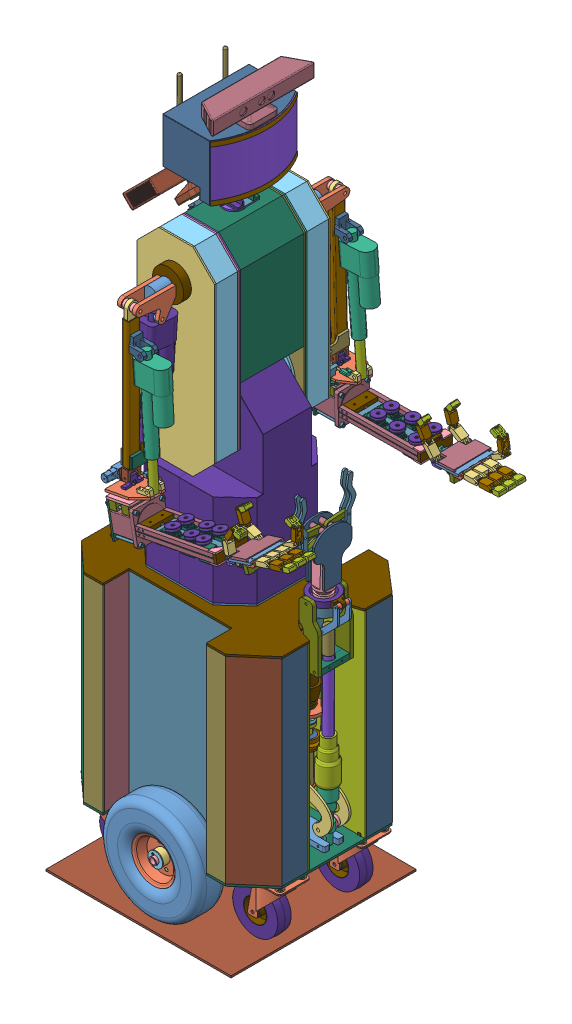
SolidWorks assembly sorbot, configuration По умолчанию. Lengths in mm. (continued)
Mates (geometry in assembly coordinates): (continued)
- Совпадение801: coincident anti-aligned: plane of ? through (-20.0648 1016.5246 -163.4875) normal (0 0 1); plane of body_tilt_axis_clamp-1 through (-20.0648 1016.5246 -163.4875) normal (0 0 -1)
- Концентричный435: concentric aligned: cylinder of body_axis-1 through (-20.0648 1016.5246 -50.7475) axis (0 0 -1) radius 10.9; cylinder of body_tilt_axis_clamp-2 through (-20.0648 1016.5246 -110.5942) axis (0 0 -1) radius 10.9
- Совпадение802: coincident anti-aligned: plane of ? through (-20.0648 1016.5246 -110.5942) normal (0 0 -1); plane of body_tilt_axis_clamp-2 through (-20.0648 1016.5246 -110.5942) normal (0 0 1)
- Концентричный436: concentric anti-aligned: cylinder of body_tilt_axis_clamp-1 through (-20.0648 1016.5246 -155.4875) axis (0 0 1) radius 20; cylinder of body_tilt_lever-1 through (-20.0648 1016.5246 -149.4875) axis (0 0 -1) radius 20
- Совпадение803: coincident anti-aligned: plane of body_tilt_axis_clamp-1 through (-20.0648 1016.5246 -155.4875) normal (0 0 1); plane of body_tilt_lever-1 through (-97.2168 978.7734 -155.4875) normal (0 0 -1)
- Заблокировать382: lock: unknown of ?; unknown of ?
- Заблокировать383: lock: unknown of ?; unknown of ?
- Заблокировать386: lock: unknown of ?; unknown of ?
- Заблокировать387: lock: unknown of ?; unknown of ?
- Заблокировать388: lock: unknown of body_pivot_fixture-1; unknown of body_pivot-2
- Заблокировать389: lock: unknown of ?; unknown of ?
- Заблокировать391: lock: unknown of body_pivot_fixture-1; unknown of ?
- Концентричный439: concentric aligned: cylinder of body_tilt_axis_clamp-2 through (-20.0648 1016.5246 -118.5942) axis (0 0 -1) radius 20; cylinder of body_tilt_lever-2 through (-20.0648 1016.5246 -118.5942) axis (0 0 -1) radius 20
- Концентричный440: concentric aligned: cylinder of body_tilt_lever-1 through (-99.3474 976.856 -149.4875) axis (0 0 -1) radius 5; cylinder of body_tilt_lever-2 through (-99.3474 976.856 -118.5942) axis (0 0 -1) radius 5
- Совпадение805: coincident anti-aligned: plane of body_tilt_axis_clamp-2 through (-20.0648 1016.5246 -118.5942) normal (0 0 -1); plane of body_tilt_lever-2 through (-97.2168 978.7734 -118.5942) normal (0 0 1)
- Концентричный441: concentric aligned: cylinder of body_tilt_lever-1 through (-99.3474 976.856 -149.4875) axis (0 0 -1) radius 5; cylinder of body_tilt_lever_axis-1 through (-99.3474 976.856 -80.4875) axis (0 0 -1) radius 5
- Расстояние22: distance = 40 mm aligned: plane of body_tilt_lever-1 through (-97.2168 978.7734 -155.4875) normal (0 0 -1); plane of body_tilt_lever_axis-1 through (-99.3474 976.856 -195.4875) normal (0 0 -1)
- Концентричный442: concentric anti-aligned: cylinder of body.tilit.lever.2-1 through (-99.3474 976.856 -188.4655) axis (0 0 1) radius 5; cylinder of body_tilt_lever_axis-1 through (-99.3474 976.856 -80.4875) axis (0 0 -1) radius 5
- Концентричный443: concentric anti-aligned: cylinder of tilt.thread.rod-1 through (-119.3768 928.5591 -141.6211) axis (0 1 0) radius 6; cylinder of body.tilt.nut-1 through (-119.3768 842.3995 -141.6211) axis (0 -1 0) radius 8
- Концентричный444: concentric anti-aligned: cylinder of tilt.thread.rod-1 through (-119.3768 928.5591 -141.6211) axis (0 1 0) radius 6; cylinder of body.tilit.nut.housing-1 through (-119.3768 838.3995 -141.6211) axis (0 -1 0) radius 8
- Концентричный445: concentric anti-aligned: cylinder of body.tilit.lever.2-1 through (-119.3768 828.3995 -188.4655) axis (0 0 1) radius 5; cylinder of body.tilit.nut.housing-1 through (-119.3768 828.3995 -156.4655) axis (0 0 -1) radius 5
- Концентричный446: concentric aligned: cylinder of body.tilit.nut.housing-1 through (-119.3768 828.3995 -156.4655) axis (0 0 -1) radius 5; cylinder of body.tilit.nut.housing.bolt-1 through (-119.3768 828.3995 -158.4655) axis (0 0 -1) radius 5
- Совпадение808: coincident anti-aligned: plane of body.tilt.nut-1 through (-110.3768 828.3995 -126.0327) normal (0 -1 0); plane of body.tilit.nut.housing-1 through (-94.3768 828.3995 -157.2211) normal (0 1 0)
- Параллельность198: parallel anti-aligned: plane of body.tilt.nut-1 through (-110.3768 842.3995 -157.2096) normal (0 0 -1); plane of body.tilit.nut.housing-1 through (-144.3768 828.3995 -157.2211) normal (0 0 1)
- Заблокировать392: lock: unknown of ?; unknown of ?
- Совпадение810: coincident anti-aligned: plane of body.tilit.lever.2-1 through (-119.3768 828.3995 -181.4655) normal (0 0 1); plane of body.tilit.nut.housing-1 through (-141.3638 838.3995 -181.4655) normal (0 0 -1)
- Совпадение811: coincident anti-aligned: plane of body.tilit.lever.2-1 through (-119.3768 828.3995 -188.4655) normal (0 0 -1); plane of body.tilit.nut.housing.bolt-1 through (-129.642 830.0202 -188.4655) normal (0 0 1)
- Концентричный447: concentric anti-aligned: cylinder of body_tilt_lever_axis-1 through (-99.3474 976.856 -80.4875) axis (0 0 -1) radius 5; cylinder of body.tilit.extender-1 through (-99.3474 976.856 -176.9875) axis (0 0 1) radius 5
- Совпадение812: coincident anti-aligned: plane of body_tilt_lever-1 through (-97.2168 978.7734 -155.4875) normal (0 0 -1); plane of body.tilit.extender-1 through (-99.3474 976.856 -155.4875) normal (0 0 1)
- Концентричный448: concentric aligned: cylinder of body_tilt_lever_axis-1 through (-99.3474 976.856 -80.4875) axis (0 0 -1) radius 5; cylinder of washer-1 through (-99.3474 976.856 -188.4655) axis (0 0 -1) radius 5
- Совпадение813: coincident anti-aligned: plane of body.tilit.lever.2-1 through (-119.3768 828.3995 -188.4655) normal (0 0 -1); plane of washer-1 through (-99.3474 976.856 -188.4655) normal (0 0 1)
- Концентричный449: concentric anti-aligned: cylinder of body_tilt_lever_axis-1 through (-99.3474 976.856 -80.4875) axis (0 0 -1) radius 5; cylinder of body.tilit.extender-2 through (-99.3474 976.856 -118.5942) axis (0 0 1) radius 5
- Совпадение814: coincident anti-aligned: plane of body_tilt_lever-2 through (-97.2168 978.7734 -118.5942) normal (0 0 1); plane of body.tilit.extender-2 through (-99.3474 976.856 -118.5942) normal (0 0 -1)
- Концентричный450: concentric anti-aligned: cylinder of body_tilt_lever_axis-1 through (-99.3474 976.856 -80.4875) axis (0 0 -1) radius 5; cylinder of body.tilit.lever.2-2 through (-99.3474 976.856 -101.7768) axis (0 0 1) radius 5
- Концентричный451: concentric aligned: cylinder of body.tilit.nut.housing-1 through (-119.3768 828.3995 -126.7768) axis (0 0 1) radius 5; cylinder of body.tilit.lever.2-2 through (-119.3768 828.3995 -101.7768) axis (0 0 1) radius 5
- Совпадение816: coincident anti-aligned: plane of body.tilit.nut.housing-1 through (-141.3638 838.3995 -101.7768) normal (0 0 1); plane of body.tilit.lever.2-2 through (-119.3768 828.3995 -101.7768) normal (0 0 -1)
- Концентричный452: concentric aligned: cylinder of body.tilit.nut.housing-1 through (-119.3768 828.3995 -126.7768) axis (0 0 1) radius 5; cylinder of body.tilit.nut.housing.bolt-2 through (-119.3768 828.3995 -124.7768) axis (0 0 1) radius 5
- Совпадение817: coincident anti-aligned: plane of body.tilit.lever.2-2 through (-119.3768 828.3995 -94.7768) normal (0 0 1); plane of body.tilit.nut.housing.bolt-2 through (-109.1117 830.0202 -94.7768) normal (0 0 -1)
- Концентричный453: concentric aligned: cylinder of body_tilt_lever_axis-1 through (-99.3474 976.856 -80.4875) axis (0 0 -1) radius 5; cylinder of washer-2 through (-99.3474 976.856 -92.7768) axis (0 0 -1) radius 5
- Совпадение818: coincident anti-aligned: plane of body.tilit.lever.2-2 through (-119.3768 828.3995 -94.7768) normal (0 0 1); plane of washer-2 through (-99.3474 976.856 -94.7768) normal (0 0 -1)
- Совпадение819: coincident anti-aligned: plane of body.frame.p1-3 through (92.5097 1436.2936 -50.7442) normal (0 0 -1); plane of arm.fixture.cap-1 through (-12.4559 1335.4922 -50.7442) normal (0 0 1)
- Совпадение820: coincident anti-aligned: plane of ? through (412.7357 1007.5295 110.4481) normal (-0.012247 -0.004016 0.999917); plane of finger.p2-10 through (405.8167 1000.5207 110.3352) normal (0.012247 0.004016 -0.999917)
- Заблокировать394: lock: unknown of ?; unknown of ?
- Заблокировать395: lock: unknown of ?; unknown of ?
- Заблокировать396: lock: unknown of ?; unknown of ?
- Заблокировать397: lock: unknown of ?; unknown of ?
- Заблокировать398: lock: unknown of ?; unknown of ?
- Заблокировать399: lock: unknown of ?; unknown of ?
- Заблокировать402: lock: unknown of ?; unknown of ?
- Заблокировать405: lock: unknown of ?; unknown of ?
- Концентричный459: concentric anti-aligned: cylinder of cap-hinge-p1-3 through (95.5097 1327.1115 -226.3787) axis (0 -1 0) radius 2; cylinder of cap-hinge-5 through (95.5097 1287.9494 -226.3787) axis (0 1 0) radius 2
- Совпадение845: coincident anti-aligned: plane of cap-hinge-p1-3 through (75.5097 1317.9494 -221.4356) normal (0 1 0); plane of cap-hinge-5 through (75.5404 1317.9494 -220.4411) normal (0 -1 0)
- Заблокировать404: lock: unknown of ?; unknown of ?
- Заблокировать406: lock: unknown of ?; unknown of ?
- Концентричный460: concentric anti-aligned: cylinder of cap-hinge-p1-4 through (95.5097 1143.936 -226.3787) axis (0 1 0) radius 2; cylinder of cap-hinge-4 through (95.5097 1183.1735 -226.3787) axis (0 -1 0) radius 2
- Совпадение847: coincident anti-aligned: plane of cap-hinge-4 through (75.5097 1173.1735 -232.2123) normal (0 -1 0); plane of cap-hinge-p1-4 through (75.4842 1173.1735 -231.2174) normal (0 1 0)
- Заблокировать407: lock: unknown of ?; unknown of ?
- Заблокировать410: lock: unknown of ?; unknown of ?
- Совпадение849: coincident anti-aligned: plane of body_pivot_fixture-1 through (-20.0648 937.0246 -136.9555) normal (0 -1 0); plane of tilit.thread.rod.bearing.fixture-1 through (-20.0648 937.0246 -136.9555) normal (0 1 0)
- Заблокировать411: lock: unknown of body_pivot_fixture-1; unknown of ?
- Параллельность199: parallel aligned: plane of wall6-3 through (267.1742 -18.2461 -216.2424) normal (1 0 0); plane of ? through (92.0581 957.5993 348.483) normal (1 0 0)
- Заблокировать412: lock: unknown of ?; unknown of ?
- Совпадение851: coincident anti-aligned: plane of body.frame.p4-4 through (-117.3772 1436.2936 -226.3595) normal (0 0 1); plane of shoulder.bearing.housing-4 through (-12.3772 1335.516 -226.3595) normal (0 0 -1)
- Концентричный462: concentric aligned: cylinder of body.frame.p4-4 through (-12.3772 1335.516 -226.3595) axis (0 0 -1) radius 12.5; cylinder of shoulder.bearing.housing-4 through (-12.3772 1335.516 -205.3595) axis (0 0 -1) radius 15.5
- Заблокировать413: lock: unknown of ?; unknown of ?
- Концентричный463: concentric aligned: cylinder of shoulder.bearing.housing-3 through (-12.6499 1335.3853 -313.3595) axis (0 0 1) radius 15.5; cylinder of shoulder.axis-2 through (-12.6499 1335.3853 -317.3595) axis (0 0 1) radius 15
- Совпадение853: coincident aligned: plane of shoulder.bearing.housing-4 through (-12.3772 1335.516 -205.3595) normal (0 0 1); plane of shoulder.axis-2 through (-12.6499 1335.3853 -205.3595) normal (0 0 1)
- Совпадение855: coincident: plane of body.frame.p4-4 through (-117.3772 1436.2936 -230.3595) normal (0 0 -1); plane of shoulder.p6-3
- Совпадение856: coincident anti-aligned: plane of shoulder.p6-4 through (-12.6499 1335.3853 -288.3595) normal (0 0 -1); plane of body.frame.p4.external-1 through (-117.6384 1436.1749 -288.3595) normal (0 0 1)
- Концентричный464: concentric aligned: cylinder of shoulder.axis-2 through (-12.6499 1335.3853 -317.3595) axis (0 0 1) radius 15; cylinder of shoulder.p6-3 through (-12.6499 1335.3853 -245.2739) axis (0 0 1) radius 15
- Концентричный465: concentric anti-aligned: cylinder of shoulder.axis-2 through (-12.6499 1335.3853 -317.3595) axis (0 0 1) radius 15; cylinder of shoulder.p6-4 through (-12.6499 1335.3853 -270.3595) axis (0 0 -1) radius 15
- Совпадение857: coincident: plane of ?; plane of shoulder.p4-3 through (-59.8188 1400.1357 -245.3595) normal (0 0 1)
- Совпадение858: coincident anti-aligned: plane of shoulder.p6-4 through (-12.6499 1335.3853 -270.3595) normal (0 0 1); plane of shoulder.p4-4 through (-59.8188 1400.1357 -270.3595) normal (0 0 -1)
- Концентричный466: concentric anti-aligned: cylinder of shoulder.axis-2 through (-12.6499 1335.3853 -317.3595) axis (0 0 1) radius 15; cylinder of shoulder.p4-4 through (-12.6499 1335.3853 -266.3595) axis (0 0 -1) radius 15
- Концентричный467: concentric anti-aligned: cylinder of shoulder.axis-2 through (-12.6499 1335.3853 -317.3595) axis (0 0 1) radius 15; cylinder of shoulder.p4-3 through (-12.6499 1335.3853 -245.3595) axis (0 0 -1) radius 15
- Совпадение865: coincident anti-aligned: plane of body.frame.p4-4 through (-117.3772 1436.2936 -230.3595) normal (0 0 -1); plane of arm.lift.actuator.fixture.p3-3 through (-88.5702 993.1387 -230.3595) normal (0 0 1)
- Концентричный469: concentric aligned: cylinder of arm.lift.actuator.fixture.p3-3 through (-88.5702 993.1387 -230.3595) axis (0 0 -1) radius 4; cylinder of arm.lift.actuator.fixture.p2-2 through (-88.5702 993.1387 -230.3595) axis (0 0 -1) radius 4
- Заблокировать416: lock: unknown of ?; unknown of ?
- Заблокировать415: lock: unknown of ?; unknown of ?
- Концентричный470: concentric anti-aligned: cylinder of arm.lift.actuator.fixture.p3-4 through (-88.5702 993.1387 -288.3595) axis (0 0 1) radius 4; cylinder of arm.lift.actuator.fixture.p2-2 through (-88.5702 993.1387 -230.3595) axis (0 0 -1) radius 4
- Концентричный478: concentric aligned: cylinder of arm.lift.actuator.fixture.p2-2 through (-88.5702 993.1387 -230.3595) axis (0 0 -1) radius 4; cylinder of arm.actuator-4/arm.actuator.p1-1 through (-88.5702 993.1387 -244.3595) axis (0 0 -1) radius 4.1
- Касательный33: tangent anti-aligned: plane of arm.lift.actuator.fixture.p3-3 through (-88.5702 993.1387 -249.3595) normal (0 0 -1); cylinder of arm.actuator-4/arm.actuator.p1-1 through (-89.1112 985.157 -259.3595) axis (0.067628 0.997711 0) radius 10
- Концентричный480: concentric anti-aligned: cylinder of arm.actuator-4/arm.actuator.p1-1 through (-79.508 1126.8319 -259.3595) axis (0.067628 0.997711 0) radius 10; cylinder of arm.actuator.p2-4 through (-60.3086 1410.0778 -259.3595) axis (-0.067628 -0.997711 0) radius 10
- Концентричный482: concentric anti-aligned: cylinder of shoulder.p4-4 through (-60.8835 1401.5972 -266.3595) axis (0 0 -1) radius 4; cylinder of arm.actuator.p2-4 through (-60.8835 1401.5972 -284.3595) axis (0 0 1) radius 4
- Концентричный481: concentric anti-aligned: cylinder of shoulder.p4-3 through (-60.8835 1401.5972 -245.3595) axis (0 0 -1) radius 4; cylinder of arm.actuator.p2-4 through (-60.8835 1401.5972 -284.3595) axis (0 0 1) radius 4
- Заблокировать418: lock: unknown of ?; unknown of ?
- Заблокировать419: lock: unknown of ?; unknown of ?
- Концентричный483: concentric anti-aligned: cylinder of arm.fixture-4 through (2.8485 1335.3868 -413.2628) axis (0.999986 0 0.005196) radius 4; cylinder of arm.lift2.actuator.fixture.p1-4 through (2.8485 1335.3868 -413.2628) axis (-0.999986 0 -0.005196) radius 4
- Совпадение869: coincident anti-aligned: plane of arm.fixture-4 through (2.8437 1335.375 -412.3468) normal (-0.999986 0 -0.005196); plane of arm.lift2.actuator.fixture.p1-4 through (2.8485 1335.3868 -413.2628) normal (0.999986 0 0.005196)
- Заблокировать420: lock: unknown of ?; unknown of ?
- Концентричный484: concentric aligned: cylinder of shoulder.lever-2 through (-7.1514 1335.3868 -413.3148) axis (-0.999986 0 -0.005196) radius 4; cylinder of arm.lift2.actuator.fixture.p1-4 through (2.8485 1335.3868 -413.2628) axis (-0.999986 0 -0.005196) radius 4
- Совпадение870: coincident anti-aligned: plane of shoulder.lever-2 through (-7.1514 1335.3868 -413.3154) normal (0.999986 0 0.005196); plane of arm.lift2.actuator.fixture.p1-4 through (-7.1514 1335.3868 -413.3148) normal (-0.999986 0 -0.005196)
- Концентричный485: concentric anti-aligned: cylinder of arm.fixture-5 through (-37.1514 1335.3868 -413.3148) axis (0.999986 0 0.005196) radius 4; cylinder of arm.lift2.actuator.fixture.p1-5 through (-17.1517 1335.3868 -413.2109) axis (-0.999986 0 -0.005196) radius 4
- Совпадение871: coincident anti-aligned: plane of arm.fixture-5 through (-27.1563 1335.375 -412.3468) normal (0.999986 0 0.005196); plane of arm.lift2.actuator.fixture.p1-5 through (-27.1515 1335.3868 -413.2628) normal (-0.999986 0 -0.005196)
- Заблокировать422: lock: unknown of ?; unknown of ?
- Концентричный486: concentric anti-aligned: cylinder of arm.fixture-4 through (2.5373 1286.6879 -353.3754) axis (0.999986 0 0.005196) radius 4; cylinder of arm.actuator-5/arm.actuator.p1-1 through (2.5373 1286.6879 -353.3754) axis (-0.999986 0 -0.005196) radius 4.1
- Концентричный487: concentric anti-aligned: cylinder of arm.fixture-4 through (2.5373 1286.6879 -353.3754) axis (0.999986 0 0.005196) radius 4; cylinder of arm.lift2.actuator.fixture.p1.m1-3 through (2.5373 1286.6879 -353.3754) axis (-0.999986 0 -0.005196) radius 4
- Совпадение873: coincident anti-aligned: plane of arm.fixture-4 through (2.8437 1335.375 -412.3468) normal (-0.999986 0 -0.005196); plane of arm.lift2.actuator.fixture.p1.m1-3 through (2.5373 1286.6879 -353.3754) normal (0.999986 0 0.005196)
- Концентричный488: concentric anti-aligned: cylinder of arm.fixture-5 through (-37.4626 1286.6879 -353.4274) axis (0.999986 0 0.005196) radius 4; cylinder of arm.lift2.actuator.fixture.p1.m1-4 through (-22.4628 1286.6879 -353.3495) axis (-0.999986 0 -0.005196) radius 4
- Совпадение874: coincident anti-aligned: plane of arm.fixture-5 through (-27.1563 1335.375 -412.3468) normal (0.999986 0 0.005196); plane of arm.lift2.actuator.fixture.p1.m1-4 through (-27.4627 1286.6879 -353.3754) normal (-0.999986 0 -0.005196)
- Касательный34: tangent anti-aligned: cylinder of arm.actuator-5/arm.actuator.p1-1 through (-12.4664 1294.6528 -352.7052) axis (0.000486 -0.995617 -0.093518) radius 10; plane of arm.lift2.actuator.fixture.p1.m1-3 through (-2.4627 1286.6879 -353.4014) normal (-0.999986 0 -0.005196)
- Заблокировать423: lock: unknown of ?; unknown of ?
- Заблокировать424: lock: unknown of ?; unknown of ?
- Заблокировать425: lock: unknown of ?; unknown of ?
- Заблокировать426: lock: unknown of ?; unknown of ?
- Заблокировать427: lock: unknown of ?; unknown of ?
- Заблокировать428: lock: unknown of ?; unknown of ?
- Заблокировать429: lock: unknown of ?; unknown of ?
- Заблокировать430: lock: unknown of ?; unknown of ?
- Концентричный493: concentric aligned: cylinder of actuator.100.fixture-2 through (30.5425 1248.8767 -435.037) axis (-0.005195 -0.022106 0.999742) radius 4; cylinder of arm.actuator100mm..p1-2 through (30.516 1248.7636 -429.924) axis (-0.005195 -0.022106 0.999742) radius 4
- Касательный35: tangent anti-aligned: plane of actuator.100.fixture-2 through (40.8098 1209.6631 -405.7286) normal (0.005195 0.022106 -0.999742); cylinder of arm.actuator100mm..p1-2 through (29.9802 1256.417 -414.7536) axis (0.057231 -0.998124 -0.021773) radius 10
- Концентричный495: concentric anti-aligned: cylinder of arm.actuator100mm..p1-2 through (35.3599 1162.5934 -416.8003) axis (0.057231 -0.998124 -0.021773) radius 10; cylinder of arm.actuator100mm.p2-2 through (49.2611 920.154 -422.0889) axis (-0.057231 0.998124 0.021773) radius 10
- Заблокировать445: lock: unknown of ?; unknown of ?
- Заблокировать446: lock: unknown of ?; unknown of ?
- Заблокировать447: lock: unknown of ?; unknown of ?
- Заблокировать448: lock: unknown of ?; unknown of ?
- Заблокировать449: lock: unknown of ?; unknown of ?
- Заблокировать450: lock: unknown of ?; unknown of ?
- Заблокировать451: lock: unknown of ?; unknown of ?
- Концентричный504: concentric anti-aligned: cylinder of HS-311 Hitec Standard Servo and Horn-12/HS-311-p2-1 through (110.806 865.1228 -440.1318) axis (-0.012385 0.99968 0.022041) radius 4.064; cylinder of lower.arm.p9-8 through (110.7286 871.3708 -439.994) axis (0.012385 -0.99968 -0.022041) radius 12
- Концентричный505: concentric anti-aligned: cylinder of HS-311 Hitec Standard Servo and Horn-8/HS-311-p2-1 through (165.824 865.856 -442.4703) axis (-0.012385 0.99968 0.022041) radius 4.064; cylinder of lower.arm.p9-10 through (165.7466 872.104 -442.3326) axis (0.012385 -0.99968 -0.022041) radius 12
- Концентричный506: concentric anti-aligned: cylinder of HS-311 Hitec Standard Servo and Horn-10/HS-311-p2-1 through (220.8415 866.5874 -444.7289) axis (-0.012385 0.99968 0.022041) radius 4.064; cylinder of lower.arm.p9-12 through (220.7641 872.8354 -444.5912) axis (0.012385 -0.99968 -0.022041) radius 12
- Концентричный507: concentric anti-aligned: cylinder of HS-311 Hitec Standard Servo and Horn-11/HS-311-p2-1 through (110.6228 864.3429 -404.8609) axis (-0.012385 0.99968 0.022041) radius 4.064; cylinder of lower.arm.p9-7 through (110.5453 870.5909 -404.7231) axis (0.012385 -0.99968 -0.022041) radius 12
- Концентричный508: concentric anti-aligned: cylinder of HS-311 Hitec Standard Servo and Horn-7/HS-311-p2-1 through (165.6133 864.9593 -401.9208) axis (-0.012385 0.99968 0.022041) radius 4.064; cylinder of lower.arm.p9-9 through (165.5359 871.2073 -401.783) axis (0.012385 -0.99968 -0.022041) radius 12
- Концентричный509: concentric anti-aligned: cylinder of HS-311 Hitec Standard Servo and Horn-9/HS-311-p2-1 through (220.6042 865.5775 -399.0607) axis (-0.012385 0.99968 0.022041) radius 4.064; cylinder of lower.arm.p9-11 through (220.5268 871.8255 -398.923) axis (0.012385 -0.99968 -0.022041) radius 12
- Совпадение938: coincident anti-aligned: plane of HS-311 Hitec Standard Servo and Horn-12/HS-311-p2-1 through (112.9596 871.5833 -448.3789) normal (-0.012385 0.99968 0.022041); plane of lower.arm.p9-8 through (110.7286 871.3708 -439.994) normal (0.012385 -0.99968 -0.022041)
- Совпадение939: coincident anti-aligned: plane of HS-311 Hitec Standard Servo and Horn-8/HS-311-p2-1 through (167.9775 872.3165 -450.7175) normal (-0.012385 0.99968 0.022041); plane of lower.arm.p9-10 through (165.7466 872.104 -442.3326) normal (0.012385 -0.99968 -0.022041)
- Совпадение940: coincident anti-aligned: plane of HS-311 Hitec Standard Servo and Horn-10/HS-311-p2-1 through (222.9951 873.0479 -452.9761) normal (-0.012385 0.99968 0.022041); plane of lower.arm.p9-12 through (220.7641 872.8354 -444.5912) normal (0.012385 -0.99968 -0.022041)
- Совпадение941: coincident anti-aligned: plane of HS-311 Hitec Standard Servo and Horn-9/HS-311-p2-1 through (222.7577 872.038 -407.3079) normal (-0.012385 0.99968 0.022041); plane of lower.arm.p9-11 through (220.5268 871.8255 -398.923) normal (0.012385 -0.99968 -0.022041)
- Совпадение942: coincident anti-aligned: plane of HS-311 Hitec Standard Servo and Horn-7/HS-311-p2-1 through (167.7668 871.4198 -410.168) normal (-0.012385 0.99968 0.022041); plane of lower.arm.p9-9 through (165.5359 871.2073 -401.783) normal (0.012385 -0.99968 -0.022041)
- Совпадение943: coincident anti-aligned: plane of HS-311 Hitec Standard Servo and Horn-11/HS-311-p2-1 through (112.7763 870.8034 -413.108) normal (-0.012385 0.99968 0.022041); plane of lower.arm.p9-7 through (110.5453 870.5909 -404.7231) normal (0.012385 -0.99968 -0.022041)
- Заблокировать452: lock: unknown of ?; unknown of ?
- Заблокировать453: lock: unknown of ?; unknown of ?
- Заблокировать454: lock: unknown of ?; unknown of ?
- Заблокировать455: lock: unknown of ?; unknown of ?
- Заблокировать456: lock: unknown of ?; unknown of ?
- Заблокировать458: lock: unknown of ?; unknown of ?
- Совпадение963: coincident anti-aligned: plane of palm.p1-4 through (362.2803 874.0257 -470.765) normal (-0.060104 0.997955 0.021755); plane of palm.p6-3 through (295.9379 868.6488 -407.401) normal (0.060104 -0.997955 -0.021755)
- Совпадение964: coincident anti-aligned: plane of palm.p1-4 through (362.2803 874.0257 -470.765) normal (-0.060104 0.997955 0.021755); plane of palm.p6-4 through (296.3955 869.3003 -436.0217) normal (0.060104 -0.997955 -0.021755)
- Совпадение965: coincident anti-aligned: plane of palm.p1-4 through (362.2803 874.0257 -470.765) normal (-0.060104 0.997955 0.021755); plane of palm.p5-3 through (330.0768 870.2924 -388.4794) normal (0.060104 -0.997955 -0.021755)
- Совпадение966: coincident anti-aligned: plane of palm.p1-4 through (362.2803 874.0257 -470.765) normal (-0.060104 0.997955 0.021755); plane of palm.p5-4 through (330.5285 871.7398 -453.6282) normal (0.060104 -0.997955 -0.021755)
- Заблокировать459: lock: unknown of ?; unknown of ?
- Заблокировать460: lock: unknown of ?; unknown of ?
- Заблокировать461: lock: unknown of ?; unknown of ?
- Заблокировать462: lock: unknown of ?; unknown of ?
- Совпадение967: coincident anti-aligned: plane of palm.p1-4 through (362.2803 874.0257 -470.765) normal (-0.060104 0.997955 0.021755); plane of palm.cap-2 through (306.1449 870.1321 -447.243) normal (0.060104 -0.997955 -0.021755)
- Совпадение968: coincident aligned: plane of palm.p1-4 through (286.8974 867.3169 -371.2793) normal (-0.998179 -0.059975 -0.006513); plane of palm.cap-2 through (286.6609 873.8329 -395.0363) normal (-0.998179 -0.059975 -0.006513)
- Совпадение969: coincident aligned: plane of palm.p1-4 through (286.8974 867.3169 -371.2793) normal (-0.005195 -0.022106 0.999742); plane of palm.cap-2 through (349.3088 877.0763 -370.7392) normal (-0.005195 -0.022106 0.999742)
- Заблокировать463: lock: unknown of ?; unknown of ?
- Совпадение970: coincident anti-aligned: plane of palm.p1-4 through (362.641 868.038 -470.8956) normal (0.060104 -0.997955 -0.021755); plane of palm.p3.m-3 through (319.6212 863.2737 -371.1987) normal (-0.060104 0.997955 0.021755)
- Совпадение971: coincident aligned: plane of palm.p1-4 through (286.8974 867.3169 -371.2793) normal (-0.005195 -0.022106 0.999742); plane of palm.p3.m-3 through (287.7592 869.3718 -371.2294) normal (-0.005195 -0.022106 0.999742)
- Совпадение972: coincident anti-aligned: plane of palm.p1-4 through (296.9 868.0051 -375.2131) normal (-0.998179 -0.059975 -0.006513); plane of palm.p3.m-3 through (296.6978 870.9282 -371.1485) normal (0.998179 0.059975 0.006513)
- Заблокировать464: lock: unknown of ?; unknown of ?
- Совпадение973: coincident anti-aligned: plane of palm.p1-4 through (362.641 868.038 -470.8956) normal (0.060104 -0.997955 -0.021755); plane of palm.p3.m-4 through (320.029 865.0091 -449.6784) normal (-0.060104 0.997955 0.021755)
- Совпадение974: coincident aligned: plane of palm.p1-4 through (287.4169 869.5276 -471.2535) normal (0.005195 0.022106 -0.999742); plane of palm.p3.m-4 through (288.2787 871.5825 -471.2036) normal (0.005195 0.022106 -0.999742)
- Совпадение975: coincident anti-aligned: plane of palm.p1-4 through (297.3779 870.0389 -467.1894) normal (-0.998179 -0.059975 -0.006513); plane of palm.p3.m-4 through (297.1057 872.6635 -449.6283) normal (0.998179 0.059975 0.006513)
- Заблокировать465: lock: unknown of ?; unknown of ?
- Совпадение976: coincident anti-aligned: plane of palm.p1-4 through (362.641 868.038 -470.8956) normal (0.060104 -0.997955 -0.021755); plane of palm.p3-2 through (343.569 866.8921 -471.02) normal (-0.060104 0.997955 0.021755)
- Совпадение977: coincident aligned: plane of palm.p1-4 through (286.8974 867.3169 -371.2793) normal (-0.005195 -0.022106 0.999742); plane of palm.p3-2 through (370.5503 875.8487 -370.6559) normal (-0.005195 -0.022106 0.999742)
- Совпадение978: coincident anti-aligned: plane of palm.p1-4 through (361.7608 871.8151 -370.7908) normal (0.998179 0.059975 0.006513); plane of palm.p3-2 through (362.07 877.5186 -470.6889) normal (-0.998179 -0.059975 -0.006513)
- Заблокировать466: lock: unknown of ?; unknown of ?
- Концентричный510: concentric aligned: cylinder of palm.p3.m-3 through (292.5129 865.4279 -371.2919) axis (0.005195 0.022106 -0.999742) radius 1.5; cylinder of finger.p1-7 through (292.5155 865.439 -371.7918) axis (0.005195 0.022106 -0.999742) radius 1.5
- Совпадение979: coincident anti-aligned: plane of palm.p3.m-3 through (282.5498 857.4215 -389.0252) normal (-0.005195 -0.022106 0.999742); plane of finger.p1-7 through (295.546 853.9979 -389.0334) normal (0.005195 0.022106 -0.999742)
- Концентричный512: concentric aligned: cylinder of finger.p2-13 through (267.069 896.9455 -371.2273) axis (0.005195 0.022106 -0.999742) radius 1.5; cylinder of finger.p1-7 through (267.069 896.9455 -371.2273) axis (0.005195 0.022106 -0.999742) radius 1.5
- Совпадение980: coincident anti-aligned: plane of finger.p1-7 through (268.2587 888.6357 -387.9091) normal (-0.005195 -0.022106 0.999742); plane of finger.p2-13 through (268.1702 885.8361 -387.9715) normal (0.005195 0.022106 -0.999742)
- Концентричный513: concentric aligned: cylinder of finger.p2-13 through (248.7323 931.3594 -370.5616) axis (0.005195 0.022106 -0.999742) radius 1.5; cylinder of finger.p3-7 through (248.7328 931.3619 -370.6745) axis (0.005195 0.022106 -0.999742) radius 1.5
- Совпадение981: coincident anti-aligned: plane of finger.p2-13 through (248.3728 922.9913 -387.2528) normal (-0.005195 -0.022106 0.999742); plane of finger.p3-7 through (238.9673 925.751 -387.2406) normal (0.005195 0.022106 -0.999742)
- Заблокировать467: lock: unknown of ?; unknown of ?
- Заблокировать468: lock: unknown of ?; unknown of ?
- Заблокировать469: lock: unknown of ?; unknown of ?
- Концентричный514: concentric aligned: cylinder of palm.p3.m-4 through (292.9207 867.1633 -449.7716) axis (0.005195 0.022106 -0.999742) radius 1.5; cylinder of finger.p1-8 through (292.9233 867.1743 -450.2715) axis (0.005195 0.022106 -0.999742) radius 1.5
- Совпадение982: coincident anti-aligned: plane of palm.p3.m-4 through (282.9576 859.1568 -467.505) normal (-0.005195 -0.022106 0.999742); plane of ? through (299.5757 857.2919 -467.4599) normal (0.005195 0.022106 -0.999742)
- Концентричный515: concentric aligned: cylinder of ? through (258.7432 888.9029 -449.9687) axis (0.005195 0.022106 -0.999742) radius 1.5; cylinder of finger.p2-14 through (258.7432 888.9029 -449.9687) axis (0.005195 0.022106 -0.999742) radius 1.5
- Концентричный516: concentric aligned: cylinder of ? through (248.5939 926.551 -449.1889) axis (0.005195 0.022106 -0.999742) radius 1.5; cylinder of finger.p3-8 through (248.5934 926.5485 -449.0761) axis (0.005195 0.022106 -0.999742) radius 1.5
- Совпадение983: coincident anti-aligned: plane of ? through (246.2216 918.2291 -453.3863) normal (0.005195 0.022106 -0.999742); plane of ? through (238.7666 920.662 -453.3712) normal (-0.005195 -0.022106 0.999742)
- Совпадение984: coincident anti-aligned: plane of ? through (262.647 881.4001 -466.6185) normal (-0.005195 -0.022106 0.999742); plane of ? through (257.2443 877.8585 -466.7249) normal (0.005195 0.022106 -0.999742)
- Заблокировать470: lock: unknown of ?; unknown of ?
- Заблокировать471: lock: unknown of ?; unknown of ?
- Заблокировать472: lock: unknown of ?; unknown of ?
- Концентричный517: concentric: cylinder of ? through (337.7337 1179.9805 -460.0065) axis (-0.005196 -0.004798 0.999975) radius 1.5; cylinder of finger.p1-9 through (337.3284 1179.6063 -382.0084) axis (-0.005196 -0.004798 0.999975) radius 1.5
- Совпадение985: coincident: plane of ? through (336.9553 1167.4295 -365.0684) normal (0.005196 0.004798 -0.999975); plane of ? through (331.3626 1168.8569 -365.0906) normal (-0.005196 -0.004798 0.999975)
- Заблокировать473: lock: unknown of ?
- Концентричный518: concentric aligned: cylinder of finger.p1-9 through (406.8614 874.0028 -392.5138) axis (-0.005195 -0.022106 0.999742) radius 1.5; cylinder of finger.p2-15 through (406.8614 874.0028 -392.5138) axis (-0.005195 -0.022106 0.999742) radius 1.5
- Совпадение986: coincident anti-aligned: plane of finger.p1-9 through (399.5598 868.6975 -376.1648) normal (0.005195 0.022106 -0.999742); plane of finger.p2-15 through (396.4589 868.5111 -376.185) normal (-0.005195 -0.022106 0.999742)
- Заблокировать474: lock: unknown of ?; unknown of ?
- Концентричный519: concentric aligned: cylinder of finger.p2-15 through (445.7903 876.3419 -392.2597) axis (-0.005195 -0.022106 0.999742) radius 1.5; cylinder of finger.p3-9 through (445.7898 876.3394 -392.1469) axis (-0.005195 -0.022106 0.999742) radius 1.5
- Совпадение987: coincident anti-aligned: plane of finger.p2-15 through (438.4887 871.0365 -375.9107) normal (0.005195 0.022106 -0.999742); plane of finger.p3-9 through (435.3879 870.8502 -375.931) normal (-0.005195 -0.022106 0.999742)
- Заблокировать475: lock: unknown of ?; unknown of ?
- Концентричный520: concentric aligned: cylinder of palm.p3-2 through (366.8103 873.7971 -470.7465) axis (-0.005195 -0.022106 0.999742) radius 1.5; cylinder of finger.p1-10 through (366.5376 872.6365 -418.2601) axis (-0.005195 -0.022106 0.999742) radius 1.5
- Совпадение988: coincident anti-aligned: plane of palm.p3-2 through (371.5201 863.0505 -401.4418) normal (0.005195 0.022106 -0.999742); plane of finger.p1-10 through (355.6635 866.6048 -401.4456) normal (-0.005195 -0.022106 0.999742)
- Заблокировать476: lock: unknown of ?; unknown of ?
- Концентричный521: concentric aligned: cylinder of finger.p1-10 through (406.9938 874.5665 -418.0072) axis (-0.005195 -0.022106 0.999742) radius 1.5; cylinder of finger.p2-16 through (406.9938 874.5665 -418.0072) axis (-0.005195 -0.022106 0.999742) radius 1.5
- Совпадение989: coincident anti-aligned: plane of finger.p1-10 through (399.6923 869.2612 -401.6582) normal (0.005195 0.022106 -0.999742); plane of finger.p2-16 through (396.5914 869.0749 -401.6784) normal (-0.005195 -0.022106 0.999742)
- Заблокировать477: lock: unknown of ?; unknown of ?
- Концентричный522: concentric aligned: cylinder of finger.p2-16 through (445.9228 876.9056 -417.7532) axis (-0.005195 -0.022106 0.999742) radius 1.5; cylinder of finger.p3-10 through (445.9222 876.9031 -417.6403) axis (-0.005195 -0.022106 0.999742) radius 1.5
- Совпадение990: coincident anti-aligned: plane of finger.p2-16 through (438.6212 871.6002 -401.4042) normal (0.005195 0.022106 -0.999742); plane of finger.p3-10 through (435.5204 871.4139 -401.4244) normal (-0.005195 -0.022106 0.999742)
- Заблокировать478: lock: unknown of ?; unknown of ?
- Концентричный523: concentric aligned: cylinder of palm.p3-2 through (366.8103 873.7971 -470.7465) axis (-0.005195 -0.022106 0.999742) radius 1.5; cylinder of finger.p1-11 through (366.67 873.2002 -443.7535) axis (-0.005195 -0.022106 0.999742) radius 1.5
- Совпадение991: coincident anti-aligned: plane of palm.p3-2 through (371.6526 863.6142 -426.9352) normal (0.005195 0.022106 -0.999742); plane of ? through (355.7959 867.1685 -426.939) normal (-0.005195 -0.022106 0.999742)
- Заблокировать479: lock: unknown of ?; unknown of ?
- Концентричный524: concentric aligned: cylinder of ? through (407.1263 875.1303 -443.5006) axis (-0.005195 -0.022106 0.999742) radius 1.5; cylinder of finger.p2-17 through (407.1263 875.1303 -443.5006) axis (-0.005195 -0.022106 0.999742) radius 1.5
- Совпадение992: coincident anti-aligned: plane of ? through (399.8247 869.8249 -427.1516) normal (0.005195 0.022106 -0.999742); plane of ? through (396.7239 869.6386 -427.1718) normal (-0.005195 -0.022106 0.999742)
- Заблокировать480: lock: unknown of ?; unknown of ?
- Концентричный525: concentric aligned: cylinder of ? through (446.0553 877.4693 -443.2466) axis (-0.005195 -0.022106 0.999742) radius 1.5; cylinder of finger.p3-11 through (446.0547 877.4668 -443.1338) axis (-0.005195 -0.022106 0.999742) radius 1.5
- Совпадение993: coincident anti-aligned: plane of ? through (438.7537 872.1639 -426.8976) normal (0.005195 0.022106 -0.999742); plane of ? through (435.6528 871.9776 -426.9178) normal (-0.005195 -0.022106 0.999742)
- Заблокировать481: lock: unknown of ?; unknown of ?
- Концентричный526: concentric: cylinder of ? through (411.4236 915.5645 -460.8923) axis (-0.005196 -0.004798 0.999975) radius 1.5; cylinder of finger.p1-12 through (411.4158 915.5573 -459.3923) axis (-0.005196 -0.004798 0.999975) radius 1.5
- Совпадение994: coincident: plane of ? through (403.6967 906.0873 -442.4774) normal (0.005196 0.004798 -0.999975); plane of ? through (403.9419 905.7906 -442.4776) normal (-0.005196 -0.004798 0.999975)
- Концентричный527: concentric aligned: cylinder of finger.p1-12 through (401.144 895.2287 -468.5938) axis (-0.005195 -0.022106 0.999742) radius 1.5; cylinder of finger.p2-18 through (401.144 895.2287 -468.5938) axis (-0.005195 -0.022106 0.999742) radius 1.5
- Совпадение995: coincident anti-aligned: plane of finger.p1-12 through (397.1815 887.0261 -452.2916) normal (0.005195 0.022106 -0.999742); plane of finger.p2-18 through (407.0548 885.0276 -452.2844) normal (-0.005195 -0.022106 0.999742)
- Концентричный528: concentric aligned: cylinder of finger.p2-18 through (395.4647 933.8042 -467.7704) axis (-0.005195 -0.022106 0.999742) radius 1.5; cylinder of finger.p3-12 through (395.4641 933.8017 -467.6575) axis (-0.005195 -0.022106 0.999742) radius 1.5
- Совпадение996: coincident anti-aligned: plane of finger.p2-18 through (400.9231 926.6758 -451.3954) normal (0.005195 0.022106 -0.999742); plane of finger.p3-12 through (406.8279 932.1468 -451.2437) normal (-0.005195 -0.022106 0.999742)
- Заблокировать482: lock: unknown of ?; unknown of ?
- Заблокировать483: lock: unknown of ?; unknown of ?
- Заблокировать484: lock: unknown of ?; unknown of ?
- Заблокировать485: lock: unknown of ?; unknown of ?
- Концентричный529: concentric aligned: cylinder of body_axis-1 through (-20.0648 1016.5246 -50.7475) axis (0 0 -1) radius 9; cylinder of bodu.tilit.axis.enforcement-1 through (-20.0648 1016.5246 -50.7475) axis (0 0 -1) radius 9
- Совпадение999: coincident aligned: plane of body_axis-1 through (-20.0648 1016.5246 -221.0975) normal (0 0 -1); plane of bodu.tilit.axis.enforcement-1 through (-20.0648 1016.5246 -221.0975) normal (0 0 -1)
- Заблокировать486: lock: unknown of ?; unknown of ?
- Заблокировать488: lock: unknown of ?; unknown of ?
- Заблокировать489: lock: unknown of ?; unknown of ?
- Заблокировать490: lock: unknown of ?; unknown of ?
- Заблокировать491: lock: unknown of ?; unknown of ?
- Заблокировать492: lock: unknown of ?; unknown of ?
- Заблокировать493: lock: unknown of ?; unknown of ?
- Совпадение1001: coincident anti-aligned: plane of m6.nut-1 through (8.0892 944.0246 -131.6914) normal (0 -1 0); plane of body_pivot_fixture-1 through (-20.0648 944.0246 -136.9555) normal (0 1 0)
- Концентричный530: concentric aligned: cylinder of ? through (8.0892 955.7352 -137.4649) axis (0 -1 0) radius 3; cylinder of ? through (8.0892 949.5246 -137.4649) axis (0 -1 0) radius 3
- Совпадение1002: coincident anti-aligned: plane of m6.nut-2 through (-6.429 944.0246 -155.8188) normal (0 -1 0); plane of body_pivot_fixture-1 through (-20.0648 944.0246 -136.9555) normal (0 1 0)
- Концентричный531: concentric aligned: cylinder of ? through (-6.429 955.7352 -161.5923) axis (0 -1 0) radius 3; cylinder of m6.nut-2 through (-6.429 949.5246 -161.5923) axis (0 -1 0) radius 3
- Совпадение1004: coincident anti-aligned: plane of m6.nut-3 through (-48.2188 944.0246 -130.6725) normal (0 -1 0); plane of body_pivot_fixture-1 through (-20.0648 944.0246 -136.9555) normal (0 1 0)
- Совпадение1005: coincident anti-aligned: plane of m6.nut-4 through (-34.583 944.0246 -155.3093) normal (0 -1 0); plane of body_pivot_fixture-1 through (-20.0648 944.0246 -136.9555) normal (0 1 0)
- Совпадение1006: coincident anti-aligned: plane of m6.nut-5 through (-5.5466 944.0246 -107.0546) normal (0 -1 0); plane of body_pivot_fixture-1 through (-20.0648 944.0246 -136.9555) normal (0 1 0)
- Совпадение1007: coincident anti-aligned: plane of m6.nut-6 through (-33.7006 944.0246 -106.5452) normal (0 -1 0); plane of body_pivot_fixture-1 through (-20.0648 944.0246 -136.9555) normal (0 1 0)
- Концентричный532: concentric aligned: cylinder of ? through (-48.2188 955.7352 -136.446) axis (0 -1 0) radius 3; cylinder of ? through (-48.2188 949.5246 -136.446) axis (0 -1 0) radius 3
- Концентричный533: concentric aligned: cylinder of ? through (-34.583 955.7352 -161.0828) axis (0 -1 0) radius 3; cylinder of m6.nut-4 through (-34.583 949.5246 -161.0828) axis (0 -1 0) radius 3
- Концентричный534: concentric aligned: cylinder of ? through (-5.5466 955.7352 -112.8281) axis (0 -1 0) radius 3; cylinder of m6.nut-5 through (-5.5466 949.5246 -112.8281) axis (0 -1 0) radius 3
- Концентричный535: concentric aligned: cylinder of ? through (-33.7006 955.7352 -112.3187) axis (0 -1 0) radius 3; cylinder of m6.nut-6 through (-33.7006 949.5246 -112.3187) axis (0 -1 0) radius 3
- Совпадение1008: coincident anti-aligned: plane of ? through (-20.0648 662.7934 -136.9555) normal (0 -1 0); plane of m6.nut-12 through (-48.2188 662.7934 -130.6725) normal (0 1 0)
- Концентричный536: concentric aligned: cylinder of ? through (-48.2188 955.7352 -136.446) axis (0 -1 0) radius 3; cylinder of ? through (-48.2188 662.7934 -136.446) axis (0 -1 0) radius 3
- Совпадение1009: coincident anti-aligned: plane of ? through (-20.0648 662.7934 -136.9555) normal (0 -1 0); plane of m6.nut-11 through (-33.7006 662.7934 -106.5452) normal (0 1 0)
- Концентричный537: concentric aligned: cylinder of ? through (-33.7006 955.7352 -112.3187) axis (0 -1 0) radius 3; cylinder of m6.nut-11 through (-33.7006 662.7934 -112.3187) axis (0 -1 0) radius 3
- Совпадение1010: coincident anti-aligned: plane of ? through (-20.0648 662.7934 -136.9555) normal (0 -1 0); plane of m6.nut-7 through (-5.5466 662.7934 -107.0546) normal (0 1 0)
- Концентричный538: concentric aligned: cylinder of ? through (-5.5466 955.7352 -112.8281) axis (0 -1 0) radius 3; cylinder of m6.nut-7 through (-5.5466 662.7934 -112.8281) axis (0 -1 0) radius 3
- Совпадение1011: coincident anti-aligned: plane of ? through (-20.0648 662.7934 -136.9555) normal (0 -1 0); plane of m6.nut-8 through (-34.583 662.7934 -155.3093) normal (0 1 0)
- Концентричный539: concentric aligned: cylinder of ? through (-34.583 955.7352 -161.0828) axis (0 -1 0) radius 3; cylinder of m6.nut-8 through (-34.583 662.7934 -161.0828) axis (0 -1 0) radius 3
- Совпадение1012: coincident anti-aligned: plane of ? through (-20.0648 662.7934 -136.9555) normal (0 -1 0); plane of m6.nut-10 through (-6.429 662.7934 -155.8188) normal (0 1 0)
- Концентричный540: concentric aligned: cylinder of ? through (-6.429 955.7352 -161.5923) axis (0 -1 0) radius 3; cylinder of m6.nut-10 through (-6.429 662.7934 -161.5923) axis (0 -1 0) radius 3
- Совпадение1013: coincident anti-aligned: plane of ? through (-20.0648 662.7934 -136.9555) normal (0 -1 0); plane of m6.nut-9 through (8.0892 662.7934 -131.6914) normal (0 1 0)
- Концентричный541: concentric aligned: cylinder of ? through (8.0892 955.7352 -137.4649) axis (0 -1 0) radius 3; cylinder of ? through (8.0892 662.7934 -137.4649) axis (0 -1 0) radius 3
- Концентричный542: concentric anti-aligned: cylinder of body_tilt_lever_axis-1 through (-99.3474 976.856 -80.4875) axis (0 0 -1) radius 5; cylinder of body.tilt.intermediate.enforce-1 through (-99.3474 976.856 -149.5942) axis (0 0 1) radius 5
- Совпадение1014: coincident anti-aligned: plane of body_tilt_lever-2 through (-97.2168 978.7734 -124.5942) normal (0 0 -1); plane of body.tilt.intermediate.enforce-1 through (-99.3474 976.856 -124.5942) normal (0 0 1)
- Заблокировать498: lock: unknown of arm.fixture.cap-2; unknown of body.frame.p1-left-1
- Заблокировать499: lock: unknown of body.tilit.enforcement-2; unknown of body.frame.p1-left-1
- Заблокировать500: lock: unknown of body.frame.p2-1; unknown of body.frame.p1-left-1
- Заблокировать501: lock: unknown of body_tilt_drive_frame_cap-1; unknown of body.frame.p3-1
- Совпадение1021: coincident anti-aligned: plane of body.frame.p1-left-1 through (92.5148 1436.2936 -222.3595) normal (0 0 1); plane of arm.drive.motor.pair-1 through (3.7745 1243.7974 -222.3595) normal (0 0 -1)
- Совпадение1022: coincident anti-aligned: plane of body.frame.p1-3 through (92.5097 1436.2936 -50.7442) normal (0 0 -1); plane of arm.drive.motor-1 through (-20.8275 1162.0905 -50.7442) normal (0 0 1)
- Концентричный547: concentric anti-aligned: cylinder of arm.actuator.p2-5 through (-12.3063 966.5653 -383.5224) axis (-0.000486 0.995617 0.093518) radius 10; cylinder of arm.actuator-5/arm.actuator.p1-1 through (-12.3974 1153.2752 -365.9848) axis (0.000486 -0.995617 -0.093518) radius 10
- Концентричный549: concentric anti-aligned: cylinder of arm.drive.p3-1 through (3.7745 1243.7974 -65.7442) axis (0 0 1) radius 6; cylinder of arm.drive.p5-1 through (3.7745 1243.7974 -50.7442) axis (0 0 -1) radius 6
- Совпадение1023: coincident anti-aligned: plane of body.frame.p1-3 through (92.5097 1436.2936 -50.7442) normal (0 0 -1); plane of arm.drive.p5-1 through (3.7745 1243.7974 -50.7442) normal (0 0 1)
- Концентричный550: concentric anti-aligned: cylinder of arm.drive.p3-1 through (3.7745 1243.7974 -65.7442) axis (0 0 1) radius 6; cylinder of arm.drive.p6-1 through (3.7745 1243.7974 -50.7442) axis (0 0 -1) radius 7
- Совпадение1024: coincident anti-aligned: plane of body.frame.p1-3 through (92.5097 1436.2936 -50.7442) normal (0 0 -1); plane of arm.drive.p6-1 through (3.7745 1243.7974 -50.7442) normal (0 0 1)
- Концентричный551: concentric anti-aligned: cylinder of arm.drive.p3-1 through (3.7745 1243.7974 -65.7442) axis (0 0 1) radius 6; cylinder of arm.drive.motor.pair-1 through (3.7745 1243.7974 -192.8595) axis (0 0 -1) radius 8
- Заблокировать504: lock: unknown of body.frame.p1-left-1; unknown of arm.drive.motor.pair-1
- Совпадение1028: coincident anti-aligned: plane of body.frame.p1-left-1 through (92.5148 1436.2936 -222.3595) normal (0 0 1); plane of arm.drive.p3-2 through (-20.8275 1162.0905 -222.3595) normal (0 0 -1)
- Концентричный553: concentric anti-aligned: cylinder of arm.drive.motor-1 through (-20.8275 1162.0905 -80.2442) axis (0 0 1) radius 8; cylinder of arm.drive.p3-2 through (-20.8275 1162.0905 -207.3595) axis (0 0 -1) radius 6
- Концентричный554: concentric anti-aligned: cylinder of arm.drive.p3-2 through (-20.8275 1162.0905 -207.3595) axis (0 0 -1) radius 6; cylinder of arm.drive.p5-2 through (-20.8275 1162.0905 -222.3595) axis (0 0 1) radius 6
- Совпадение1029: coincident anti-aligned: plane of body.frame.p1-left-1 through (92.5148 1436.2936 -222.3595) normal (0 0 1); plane of arm.drive.p5-2 through (-20.8275 1162.0905 -222.3595) normal (0 0 -1)
- Совпадение1030: coincident anti-aligned: plane of body.frame.p1-left-1 through (92.5148 1436.2936 -222.3595) normal (0 0 1); plane of arm.drive.p6-2 through (-20.8275 1162.0905 -222.3595) normal (0 0 -1)
